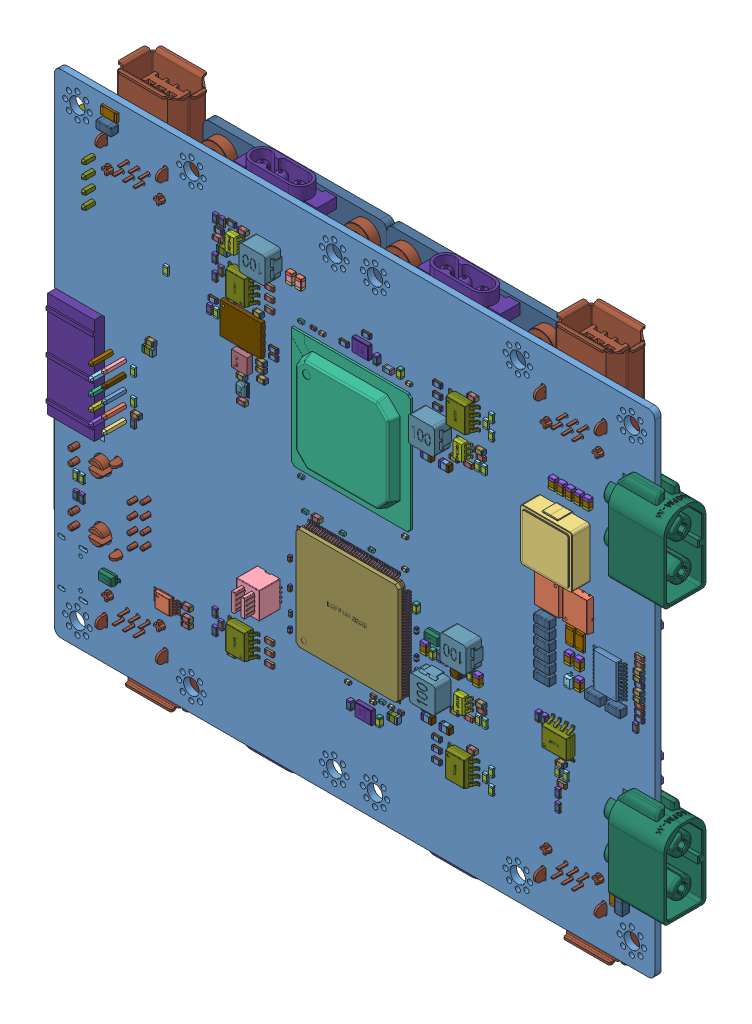
SolidWorks assembly Mother  Board, configuration 默认. Lengths in mm. (continued)
Components (placement in the parent): (continued)
- Mother  Board.step-1: Mother  Board.step [默认] at origin size (122.6 102.08 21) (continued)
  - Free-Models.step-1: Free-Models.step [默认] at origin size (70.87 98.07 8.62) (continued)
    - Driver_Board.step-4: Driver_Board.step [默认] at (21.971 0 -6.2) x (1 0 0) z (0 0 1) size (35.43 49.03 8.62) (continued)
      - R2.step-1: R2.step [默认] at origin size (0.8 1.6 0.45) (continued)
        - 6547515376.step-1: 6547515376.step [默认] at (-0.7621 21.0821 0) x (0 1 0) z (0 0 1) size (1.6 0.8 0.45) (continued)
          - Terminal-19.step-1: Terminal-19.step [默认] at (-0.8 -0.4 0) size (0.3 0.8 0.45)
            - Open_CASCADE_STEP_translator_6.8_21.2.1-76.step-1: Open_CASCADE_STEP_translator_6.8_21.2.1-76.step [默认] at origin size (0.3 0.8 0.45)
          - Terminal-19.step-2: Terminal-19.step [默认] at (0.8 0.4 0) x (-1 0 0) z (0 0 1) size (0.3 0.8 0.45)
            - Open_CASCADE_STEP_translator_6.8_21.2.1-76.step-1: Open_CASCADE_STEP_translator_6.8_21.2.1-76.step [默认] at origin size (0.3 0.8 0.45)
          - Mid_Body-77.step-1: Mid_Body-77.step [默认] at (-0.8 -0.4 0) size (1.51 0.8 0.36)
          - Mark-78.step-1: Mark-78.step [默认] at (-0.5 -0.4 0.405) size (1 0.8 0.05)
      - R1.step-1: R1.step [默认] at origin size (0.8 1.6 0.45)
        - 6547515376.step-1: 6547515376.step [默认] at (3.5559 13.5891 0) x (0 1 0) z (0 0 1) size (1.6 0.8 0.45)
          - Terminal-19.step-1: Terminal-19.step [默认] at (-0.8 -0.4 0) size (0.3 0.8 0.45)
            - Open_CASCADE_STEP_translator_6.8_21.2.1-76.step-1: Open_CASCADE_STEP_translator_6.8_21.2.1-76.step [默认] at origin size (0.3 0.8 0.45)
          - Terminal-19.step-2: Terminal-19.step [默认] at (0.8 0.4 0) x (-1 0 0) z (0 0 1) size (0.3 0.8 0.45)
            - Open_CASCADE_STEP_translator_6.8_21.2.1-76.step-1: Open_CASCADE_STEP_translator_6.8_21.2.1-76.step [默认] at origin size (0.3 0.8 0.45)
          - Mid_Body-77.step-1: Mid_Body-77.step [默认] at (-0.8 -0.4 0) size (1.51 0.8 0.36)
          - Mark-78.step-1: Mark-78.step [默认] at (-0.5 -0.4 0.405) size (1 0.8 0.05)
      - M6.step-1: M6.step [默认] at origin size (5.15 6.15 1.1)
        - TDSON-8-91.step-1: TDSON-8-91.step [默认] at (21.8441 12.7711 -1.6164) x (1 0 0) z (0 1 0) size (5.15 1.1 6.15)
      - M5.step-1: M5.step [默认] at origin size (5.15 6.15 1.1)
        - TDSON-8-91.step-1: TDSON-8-91.step [默认] at (27.3049 12.7713 -1.6164) x (-1 0 0) z (0 -1 0) size (5.15 1.1 6.15)
      - M4.step-1: M4.step [默认] at origin size (5.15 6.15 1.1)
        - TDSON-8-91.step-1: TDSON-8-91.step [默认] at (10.9221 15.0571 -1.6164) x (1 0 0) z (0 1 0) size (5.15 1.1 6.15)
      - M3.step-1: M3.step [默认] at origin size (5.15 6.15 1.1)
        - TDSON-8-91.step-1: TDSON-8-91.step [默认] at (16.3829 15.0573 -1.6164) x (-1 0 0) z (0 -1 0) size (5.15 1.1 6.15)
      - M2-1.step-1: M2-1.step [默认] at origin size (5.15 6.15 1.1)
        - TDSON-8-91.step-1: TDSON-8-91.step [默认] at (0 12.7711 -1.6164) x (1 0 0) z (0 1 0) size (5.15 1.1 6.15)
      - M1-1.step-1: M1-1.step [默认] at origin size (5.15 6.15 1.1)
        - TDSON-8-91.step-1: TDSON-8-91.step [默认] at (5.4609 12.7713 -1.6164) x (-1 0 0) z (0 -1 0) size (5.15 1.1 6.15)
      - JP4-1.step-1: JP4-1.step [默认] at origin size (5.56 5.56 4.53)
        - User_Library-SMTSO-M3-3ET.step-1: User_Library-SMTSO-M3-3ET.step [默认] at (27.5589 0.0001 -2.6164) x (0 0 1) z (0 1 0) size (4.53 5.56 5.56)
      - JP3-1.step-1: JP3-1.step [默认] at origin size (5.56 5.56 4.53)
        - User_Library-SMTSO-M3-3ET.step-1: User_Library-SMTSO-M3-3ET.step [默认] at (-0.0001 0.0001 -2.6164) x (0 0 1) z (0 1 0) size (4.53 5.56 5.56)
      - JP2.step-1: JP2.step [默认] at origin size (11.5 4.96 6.5)
        - SG340-GxxP-B1-2x12.step-1: SG340-GxxP-B1-2x12.step [默认] at (13.7793 38.9891 0) x (-1 0 0) z (0 0 1) size (11.5 4.96 6.5)
      - D3-1.step-1: D3-1.step [默认] at origin size (2.65 1.3 0.96)
        - SOD-323-1.step-1: SOD-323-1.step [默认] at (20.5836 25.1426 0.05) x (-1 0 0) z (0 0 1) size (2.65 1.3 0.96)
          - SOD-323-92.step-1: SOD-323-92.step [默认] at origin size (2.65 1.3 0.95)
          - LOGO______.__-93.step-1: LOGO______.__-93.step [默认] at (0.0033 0.0815 -0.003) x (-1 0 0) z (0 0 -1) size (0.9 1.04 0.01)
      - D2-1.step-1: D2-1.step [默认] at origin size (2.65 1.3 0.96)
        - SOD-323-1.step-1: SOD-323-1.step [默认] at (13.4716 25.1426 0.05) x (-1 0 0) z (0 0 1) size (2.65 1.3 0.96)
          - SOD-323-92.step-1: SOD-323-92.step [默认] at origin size (2.65 1.3 0.95)
          - LOGO______.__-93.step-1: LOGO______.__-93.step [默认] at (0.0033 0.0815 -0.003) x (-1 0 0) z (0 0 -1) size (0.9 1.04 0.01)
      - D1-1.step-1: D1-1.step [默认] at origin size (2.65 1.3 0.96)
        - SOD-323-1.step-1: SOD-323-1.step [默认] at (6.3596 25.1426 0.05) x (-1 0 0) z (0 0 1) size (2.65 1.3 0.96)
          - SOD-323-92.step-1: SOD-323-92.step [默认] at origin size (2.65 1.3 0.95)
          - LOGO______.__-93.step-1: LOGO______.__-93.step [默认] at (0.0033 0.0815 -0.003) x (-1 0 0) z (0 0 -1) size (0.9 1.04 0.01)
      - CP7-1.step-1: CP7-1.step [默认] at origin size (1.5 3 1.5)
        - (______)-94.step-1: (______)-94.step [默认] at (29.2101 17.1449 0) x (1 0 0) z (0 0 1) size (1.5 3 1.5)
      - CP9.step-1: CP9.step [默认] at origin size (1.5 3 1.5)
        - (______)-94.step-1: (______)-94.step [默认] at (18.2881 19.4309 0) x (1 0 0) z (0 0 1) size (1.5 3 1.5)
      - CP8-1.step-1: CP8-1.step [默认] at origin size (1.5 3 1.5)
        - (______)-94.step-1: (______)-94.step [默认] at (20.1931 19.4309 0) x (1 0 0) z (0 0 1) size (1.5 3 1.5)
      - CP5-1.step-1: CP5-1.step [默认] at origin size (1.5 3 1.5)
        - (______)-94.step-1: (______)-94.step [默认] at (9.3982 17.145 0) x (1 0 0) z (0 0 1) size (1.5 3 1.5)
      - CP4-1.step-1: CP4-1.step [默认] at origin size (1.5 3 1.5)
        - (______)-94.step-1: (______)-94.step [默认] at (7.4932 17.145 0) x (1 0 0) z (0 0 1) size (1.5 3 1.5)
      - CP3-1.step-1: CP3-1.step [默认] at origin size (1.5 3 1.5)
        - (______)-94.step-1: (______)-94.step [默认] at (27.3051 17.1449 0) x (1 0 0) z (0 0 1) size (1.5 3 1.5)
      - CP2-1.step-1: CP2-1.step [默认] at origin size (1.5 3 1.5)
        - (______)-94.step-1: (______)-94.step [默认] at (16.3831 19.4309 0) x (1 0 0) z (0 0 1) size (1.5 3 1.5)
      - CP1-1.step-1: CP1-1.step [默认] at origin size (1.5 3 1.5)
        - (______)-94.step-1: (______)-94.step [默认] at (5.5882 17.145 0) x (1 0 0) z (0 0 1) size (1.5 3 1.5)
      - C29-1.step-1: C29-1.step [默认] at origin size (1.6 0.8 0.8)
        - 6547515616.step-1: 6547515616.step [默认] at (22.9869 16.6369 0) x (-1 0 0) z (0 0 1) size (1.6 0.8 0.8)
          - Terminal-22.step-1: Terminal-22.step [默认] at (-0.8 -0.4 0) size (1.6 0.8 0.8)
            - Open_CASCADE_STEP_translator_6.8_47.1.1-85.step-1: Open_CASCADE_STEP_translator_6.8_47.1.1-85.step [默认] at origin size (0.3 0.8 0.8)
            - Open_CASCADE_STEP_translator_6.8_47.1.2-86.step-1: Open_CASCADE_STEP_translator_6.8_47.1.2-86.step [默认] at origin size (0.3 0.8 0.8)
          - Mid_Body-10.step-1: Mid_Body-10.step [默认] at (-0.8 -0.4 0) size (1 0.8 0.8)
            - Open_CASCADE_STEP_translator_6.8_47.2.1-87.step-1: Open_CASCADE_STEP_translator_6.8_47.2.1-87.step [默认] at origin size (1 0.8 0.8)
      - C28-1.step-1: C28-1.step [默认] at origin size (1.6 0.8 0.8)
        - 6547515616.step-1: 6547515616.step [默认] at (24.6379 10.6679 0) x (-1 0 0) z (0 0 1) size (1.6 0.8 0.8)
          - Terminal-22.step-1: Terminal-22.step [默认] at (-0.8 -0.4 0) size (1.6 0.8 0.8)
            - Open_CASCADE_STEP_translator_6.8_47.1.1-85.step-1: Open_CASCADE_STEP_translator_6.8_47.1.1-85.step [默认] at origin size (0.3 0.8 0.8)
            - Open_CASCADE_STEP_translator_6.8_47.1.2-86.step-1: Open_CASCADE_STEP_translator_6.8_47.1.2-86.step [默认] at origin size (0.3 0.8 0.8)
          - Mid_Body-10.step-1: Mid_Body-10.step [默认] at (-0.8 -0.4 0) size (1 0.8 0.8)
            - Open_CASCADE_STEP_translator_6.8_47.2.1-87.step-1: Open_CASCADE_STEP_translator_6.8_47.2.1-87.step [默认] at origin size (1 0.8 0.8)
      - C27-1.step-1: C27-1.step [默认] at origin size (2.01 1.25 0.94)
        - 6547513136.step-1: 6547513136.step [默认] at (20.8503 23.4725 0) x (-1 0 0) z (0 0 1) size (2.01 1.25 0.94)
          - Fillet1-95.step-1: Fillet1-95.step [默认] at origin size (0.5 1.25 0.94)
          - Fillet2-96.step-1: Fillet2-96.step [默认] at origin size (0.5 1.25 0.94)
          - body2-97.step-1: body2-97.step [默认] at origin size (1.01 1.22 0.92)
      - C26-1.step-1: C26-1.step [默认] at origin size (0.8 1.6 0.8)
        - 6547516096.step-1: 6547516096.step [默认] at (17.9295 24.7425 0) x (0 -1 0) z (0 0 1) size (1.6 0.8 0.8)
          - Terminal-23.step-1: Terminal-23.step [默认] at (-0.8 -0.4 0) size (1.6 0.8 0.8)
            - Open_CASCADE_STEP_translator_6.8_47.1.1-98.step-1: Open_CASCADE_STEP_translator_6.8_47.1.1-98.step [默认] at origin size (0.3 0.8 0.8)
            - Open_CASCADE_STEP_translator_6.8_47.1.2-99.step-1: Open_CASCADE_STEP_translator_6.8_47.1.2-99.step [默认] at origin size (0.3 0.8 0.8)
          - Mid_Body-11.step-1: Mid_Body-11.step [默认] at (-0.8 -0.4 0) size (1 0.8 0.8)
            - Open_CASCADE_STEP_translator_6.8_47.2.1-100.step-1: Open_CASCADE_STEP_translator_6.8_47.2.1-100.step [默认] at origin size (1 0.8 0.8)
      - C25-1.step-1: C25-1.step [默认] at origin size (1.25 2.01 0.94)
        - 6547514896.step-1: 6547514896.step [默认] at (23.5173 31.0126 0) x (0 1 0) z (0 0 1) size (2.01 1.25 0.94)
          - Fillet1-101.step-1: Fillet1-101.step [默认] at origin size (0.5 1.25 0.94)
          - Fillet2-102.step-1: Fillet2-102.step [默认] at origin size (0.5 1.25 0.94)
          - body2-103.step-1: body2-103.step [默认] at origin size (1.01 1.22 0.92)
      - C20-1.step-1: C20-1.step [默认] at origin size (1.6 0.8 0.8)
        - 6547515616.step-1: 6547515616.step [默认] at (12.0649 18.9229 0) x (-1 0 0) z (0 0 1) size (1.6 0.8 0.8)
          - Terminal-22.step-1: Terminal-22.step [默认] at (-0.8 -0.4 0) size (1.6 0.8 0.8)
            - Open_CASCADE_STEP_translator_6.8_47.1.1-85.step-1: Open_CASCADE_STEP_translator_6.8_47.1.1-85.step [默认] at origin size (0.3 0.8 0.8)
            - Open_CASCADE_STEP_translator_6.8_47.1.2-86.step-1: Open_CASCADE_STEP_translator_6.8_47.1.2-86.step [默认] at origin size (0.3 0.8 0.8)
          - Mid_Body-10.step-1: Mid_Body-10.step [默认] at (-0.8 -0.4 0) size (1 0.8 0.8)
            - Open_CASCADE_STEP_translator_6.8_47.2.1-87.step-1: Open_CASCADE_STEP_translator_6.8_47.2.1-87.step [默认] at origin size (1 0.8 0.8)
      - C19-1.step-1: C19-1.step [默认] at origin size (0.8 1.6 0.8)
        - 6547517776.step-1: 6547517776.step [默认] at (25.7809 37.7191 0) x (0 1 0) z (0 0 1) size (1.6 0.8 0.8)
          - Terminal-24.step-1: Terminal-24.step [默认] at (-0.8 -0.4 0) size (1.6 0.8 0.8)
            - Open_CASCADE_STEP_translator_6.8_47.1.1-104.step-1: Open_CASCADE_STEP_translator_6.8_47.1.1-104.step [默认] at origin size (0.3 0.8 0.8)
            - Open_CASCADE_STEP_translator_6.8_47.1.2-105.step-1: Open_CASCADE_STEP_translator_6.8_47.1.2-105.step [默认] at origin size (0.3 0.8 0.8)
          - Mid_Body-12.step-1: Mid_Body-12.step [默认] at (-0.8 -0.4 0) size (1 0.8 0.8)
            - Open_CASCADE_STEP_translator_6.8_47.2.1-106.step-1: Open_CASCADE_STEP_translator_6.8_47.2.1-106.step [默认] at origin size (1 0.8 0.8)
      - C18-1.step-1: C18-1.step [默认] at origin size (0.8 1.6 0.8)
        - 6547517776.step-1: 6547517776.step [默认] at (24.6379 37.7191 0) x (0 1 0) z (0 0 1) size (1.6 0.8 0.8)
          - Terminal-24.step-1: Terminal-24.step [默认] at (-0.8 -0.4 0) size (1.6 0.8 0.8)
            - Open_CASCADE_STEP_translator_6.8_47.1.1-104.step-1: Open_CASCADE_STEP_translator_6.8_47.1.1-104.step [默认] at origin size (0.3 0.8 0.8)
            - Open_CASCADE_STEP_translator_6.8_47.1.2-105.step-1: Open_CASCADE_STEP_translator_6.8_47.1.2-105.step [默认] at origin size (0.3 0.8 0.8)
          - Mid_Body-12.step-1: Mid_Body-12.step [默认] at (-0.8 -0.4 0) size (1 0.8 0.8)
            - Open_CASCADE_STEP_translator_6.8_47.2.1-106.step-1: Open_CASCADE_STEP_translator_6.8_47.2.1-106.step [默认] at origin size (1 0.8 0.8)
      - C17-1.step-1: C17-1.step [默认] at origin size (1.6 0.8 0.8)
        - 6547515616.step-1: 6547515616.step [默认] at (13.7159 12.9539 0) x (-1 0 0) z (0 0 1) size (1.6 0.8 0.8)
          - Terminal-22.step-1: Terminal-22.step [默认] at (-0.8 -0.4 0) size (1.6 0.8 0.8)
            - Open_CASCADE_STEP_translator_6.8_47.1.1-85.step-1: Open_CASCADE_STEP_translator_6.8_47.1.1-85.step [默认] at origin size (0.3 0.8 0.8)
            - Open_CASCADE_STEP_translator_6.8_47.1.2-86.step-1: Open_CASCADE_STEP_translator_6.8_47.1.2-86.step [默认] at origin size (0.3 0.8 0.8)
          - Mid_Body-10.step-1: Mid_Body-10.step [默认] at (-0.8 -0.4 0) size (1 0.8 0.8)
            - Open_CASCADE_STEP_translator_6.8_47.2.1-87.step-1: Open_CASCADE_STEP_translator_6.8_47.2.1-87.step [默认] at origin size (1 0.8 0.8)
      - C16-1.step-1: C16-1.step [默认] at origin size (0.8 1.6 0.8)
        - 6547516096.step-1: 6547516096.step [默认] at (25.7811 22.2249 0) x (0 -1 0) z (0 0 1) size (1.6 0.8 0.8)
          - Terminal-23.step-1: Terminal-23.step [默认] at (-0.8 -0.4 0) size (1.6 0.8 0.8)
            - Open_CASCADE_STEP_translator_6.8_47.1.1-98.step-1: Open_CASCADE_STEP_translator_6.8_47.1.1-98.step [默认] at origin size (0.3 0.8 0.8)
            - Open_CASCADE_STEP_translator_6.8_47.1.2-99.step-1: Open_CASCADE_STEP_translator_6.8_47.1.2-99.step [默认] at origin size (0.3 0.8 0.8)
          - Mid_Body-11.step-1: Mid_Body-11.step [默认] at (-0.8 -0.4 0) size (1 0.8 0.8)
            - Open_CASCADE_STEP_translator_6.8_47.2.1-100.step-1: Open_CASCADE_STEP_translator_6.8_47.2.1-100.step [默认] at origin size (1 0.8 0.8)
      - C15-1.step-1: C15-1.step [默认] at origin size (0.8 1.6 0.8)
        - 6547517776.step-1: 6547517776.step [默认] at (23.8759 25.6541 0) x (0 1 0) z (0 0 1) size (1.6 0.8 0.8)
          - Terminal-24.step-1: Terminal-24.step [默认] at (-0.8 -0.4 0) size (1.6 0.8 0.8)
            - Open_CASCADE_STEP_translator_6.8_47.1.1-104.step-1: Open_CASCADE_STEP_translator_6.8_47.1.1-104.step [默认] at origin size (0.3 0.8 0.8)
            - Open_CASCADE_STEP_translator_6.8_47.1.2-105.step-1: Open_CASCADE_STEP_translator_6.8_47.1.2-105.step [默认] at origin size (0.3 0.8 0.8)
          - Mid_Body-12.step-1: Mid_Body-12.step [默认] at (-0.8 -0.4 0) size (1 0.8 0.8)
            - Open_CASCADE_STEP_translator_6.8_47.2.1-106.step-1: Open_CASCADE_STEP_translator_6.8_47.2.1-106.step [默认] at origin size (1 0.8 0.8)
      - C14-1.step-1: C14-1.step [默认] at origin size (2.01 1.25 0.94)
        - 6547513136.step-1: 6547513136.step [默认] at (13.7383 23.4725 0) x (-1 0 0) z (0 0 1) size (2.01 1.25 0.94)
          - Fillet1-95.step-1: Fillet1-95.step [默认] at origin size (0.5 1.25 0.94)
          - Fillet2-96.step-1: Fillet2-96.step [默认] at origin size (0.5 1.25 0.94)
          - body2-97.step-1: body2-97.step [默认] at origin size (1.01 1.22 0.92)
      - C13-1.step-1: C13-1.step [默认] at origin size (0.8 1.6 0.8)
        - 6547516096.step-1: 6547516096.step [默认] at (10.8175 24.7425 0) x (0 -1 0) z (0 0 1) size (1.6 0.8 0.8)
          - Terminal-23.step-1: Terminal-23.step [默认] at (-0.8 -0.4 0) size (1.6 0.8 0.8)
            - Open_CASCADE_STEP_translator_6.8_47.1.1-98.step-1: Open_CASCADE_STEP_translator_6.8_47.1.1-98.step [默认] at origin size (0.3 0.8 0.8)
            - Open_CASCADE_STEP_translator_6.8_47.1.2-99.step-1: Open_CASCADE_STEP_translator_6.8_47.1.2-99.step [默认] at origin size (0.3 0.8 0.8)
          - Mid_Body-11.step-1: Mid_Body-11.step [默认] at (-0.8 -0.4 0) size (1 0.8 0.8)
            - Open_CASCADE_STEP_translator_6.8_47.2.1-100.step-1: Open_CASCADE_STEP_translator_6.8_47.2.1-100.step [默认] at origin size (1 0.8 0.8)
      - C12-1.step-1: C12-1.step [默认] at origin size (1.25 2.01 0.94)
        - 6547514896.step-1: 6547514896.step [默认] at (16.4053 31.0126 0) x (0 1 0) z (0 0 1) size (2.01 1.25 0.94)
          - Fillet1-101.step-1: Fillet1-101.step [默认] at origin size (0.5 1.25 0.94)
          - Fillet2-102.step-1: Fillet2-102.step [默认] at origin size (0.5 1.25 0.94)
          - body2-103.step-1: body2-103.step [默认] at origin size (1.01 1.22 0.92)
      - C11-1.step-1: C11-1.step [默认] at origin size (1.6 0.8 0.8)
        - 6547515616.step-1: 6547515616.step [默认] at (27.6859 22.8599 0) x (-1 0 0) z (0 0 1) size (1.6 0.8 0.8)
          - Terminal-22.step-1: Terminal-22.step [默认] at (-0.8 -0.4 0) size (1.6 0.8 0.8)
            - Open_CASCADE_STEP_translator_6.8_47.1.1-85.step-1: Open_CASCADE_STEP_translator_6.8_47.1.1-85.step [默认] at origin size (0.3 0.8 0.8)
            - Open_CASCADE_STEP_translator_6.8_47.1.2-86.step-1: Open_CASCADE_STEP_translator_6.8_47.1.2-86.step [默认] at origin size (0.3 0.8 0.8)
          - Mid_Body-10.step-1: Mid_Body-10.step [默认] at (-0.8 -0.4 0) size (1 0.8 0.8)
            - Open_CASCADE_STEP_translator_6.8_47.2.1-87.step-1: Open_CASCADE_STEP_translator_6.8_47.2.1-87.step [默认] at origin size (1 0.8 0.8)
      - C10-1.step-1: C10-1.step [默认] at origin size (0.8 1.6 0.8)
        - 6547517776.step-1: 6547517776.step [默认] at (-3.1751 37.7191 0) x (0 1 0) z (0 0 1) size (1.6 0.8 0.8)
          - Terminal-24.step-1: Terminal-24.step [默认] at (-0.8 -0.4 0) size (1.6 0.8 0.8)
            - Open_CASCADE_STEP_translator_6.8_47.1.1-104.step-1: Open_CASCADE_STEP_translator_6.8_47.1.1-104.step [默认] at origin size (0.3 0.8 0.8)
            - Open_CASCADE_STEP_translator_6.8_47.1.2-105.step-1: Open_CASCADE_STEP_translator_6.8_47.1.2-105.step [默认] at origin size (0.3 0.8 0.8)
          - Mid_Body-12.step-1: Mid_Body-12.step [默认] at (-0.8 -0.4 0) size (1 0.8 0.8)
            - Open_CASCADE_STEP_translator_6.8_47.2.1-106.step-1: Open_CASCADE_STEP_translator_6.8_47.2.1-106.step [默认] at origin size (1 0.8 0.8)
      - C9-1.step-1: C9-1.step [默认] at origin size (0.8 1.6 0.8)
        - 6547516096.step-1: 6547516096.step [默认] at (-3.1749 22.2249 0) x (0 -1 0) z (0 0 1) size (1.6 0.8 0.8)
          - Terminal-23.step-1: Terminal-23.step [默认] at (-0.8 -0.4 0) size (1.6 0.8 0.8)
            - Open_CASCADE_STEP_translator_6.8_47.1.1-98.step-1: Open_CASCADE_STEP_translator_6.8_47.1.1-98.step [默认] at origin size (0.3 0.8 0.8)
            - Open_CASCADE_STEP_translator_6.8_47.1.2-99.step-1: Open_CASCADE_STEP_translator_6.8_47.1.2-99.step [默认] at origin size (0.3 0.8 0.8)
          - Mid_Body-11.step-1: Mid_Body-11.step [默认] at (-0.8 -0.4 0) size (1 0.8 0.8)
            - Open_CASCADE_STEP_translator_6.8_47.2.1-100.step-1: Open_CASCADE_STEP_translator_6.8_47.2.1-100.step [默认] at origin size (1 0.8 0.8)
      - C8-1.step-1: C8-1.step [默认] at origin size (1.6 0.8 0.8)
        - 6547515616.step-1: 6547515616.step [默认] at (1.1429 16.5099 0) x (-1 0 0) z (0 0 1) size (1.6 0.8 0.8)
          - Terminal-22.step-1: Terminal-22.step [默认] at (-0.8 -0.4 0) size (1.6 0.8 0.8)
            - Open_CASCADE_STEP_translator_6.8_47.1.1-85.step-1: Open_CASCADE_STEP_translator_6.8_47.1.1-85.step [默认] at origin size (0.3 0.8 0.8)
            - Open_CASCADE_STEP_translator_6.8_47.1.2-86.step-1: Open_CASCADE_STEP_translator_6.8_47.1.2-86.step [默认] at origin size (0.3 0.8 0.8)
          - Mid_Body-10.step-1: Mid_Body-10.step [默认] at (-0.8 -0.4 0) size (1 0.8 0.8)
            - Open_CASCADE_STEP_translator_6.8_47.2.1-87.step-1: Open_CASCADE_STEP_translator_6.8_47.2.1-87.step [默认] at origin size (1 0.8 0.8)
      - C7-1.step-1: C7-1.step [默认] at origin size (0.8 1.6 0.8)
        - 6547516096.step-1: 6547516096.step [默认] at (-2.0319 22.2249 0) x (0 -1 0) z (0 0 1) size (1.6 0.8 0.8)
          - Terminal-23.step-1: Terminal-23.step [默认] at (-0.8 -0.4 0) size (1.6 0.8 0.8)
            - Open_CASCADE_STEP_translator_6.8_47.1.1-98.step-1: Open_CASCADE_STEP_translator_6.8_47.1.1-98.step [默认] at origin size (0.3 0.8 0.8)
            - Open_CASCADE_STEP_translator_6.8_47.1.2-99.step-1: Open_CASCADE_STEP_translator_6.8_47.1.2-99.step [默认] at origin size (0.3 0.8 0.8)
          - Mid_Body-11.step-1: Mid_Body-11.step [默认] at (-0.8 -0.4 0) size (1 0.8 0.8)
            - Open_CASCADE_STEP_translator_6.8_47.2.1-100.step-1: Open_CASCADE_STEP_translator_6.8_47.2.1-100.step [默认] at origin size (1 0.8 0.8)
      - C6-1.step-1: C6-1.step [默认] at origin size (0.8 1.6 0.8)
        - 6547517776.step-1: 6547517776.step [默认] at (-2.0321 37.7191 0) x (0 1 0) z (0 0 1) size (1.6 0.8 0.8)
          - Terminal-24.step-1: Terminal-24.step [默认] at (-0.8 -0.4 0) size (1.6 0.8 0.8)
            - Open_CASCADE_STEP_translator_6.8_47.1.1-104.step-1: Open_CASCADE_STEP_translator_6.8_47.1.1-104.step [默认] at origin size (0.3 0.8 0.8)
            - Open_CASCADE_STEP_translator_6.8_47.1.2-105.step-1: Open_CASCADE_STEP_translator_6.8_47.1.2-105.step [默认] at origin size (0.3 0.8 0.8)
          - Mid_Body-12.step-1: Mid_Body-12.step [默认] at (-0.8 -0.4 0) size (1 0.8 0.8)
            - Open_CASCADE_STEP_translator_6.8_47.2.1-106.step-1: Open_CASCADE_STEP_translator_6.8_47.2.1-106.step [默认] at origin size (1 0.8 0.8)
      - C5-1.step-1: C5-1.step [默认] at origin size (1.6 0.8 0.8)
        - 6547515616.step-1: 6547515616.step [默认] at (2.7939 10.6679 0) x (-1 0 0) z (0 0 1) size (1.6 0.8 0.8)
          - Terminal-22.step-1: Terminal-22.step [默认] at (-0.8 -0.4 0) size (1.6 0.8 0.8)
            - Open_CASCADE_STEP_translator_6.8_47.1.1-85.step-1: Open_CASCADE_STEP_translator_6.8_47.1.1-85.step [默认] at origin size (0.3 0.8 0.8)
            - Open_CASCADE_STEP_translator_6.8_47.1.2-86.step-1: Open_CASCADE_STEP_translator_6.8_47.1.2-86.step [默认] at origin size (0.3 0.8 0.8)
          - Mid_Body-10.step-1: Mid_Body-10.step [默认] at (-0.8 -0.4 0) size (1 0.8 0.8)
            - Open_CASCADE_STEP_translator_6.8_47.2.1-87.step-1: Open_CASCADE_STEP_translator_6.8_47.2.1-87.step [默认] at origin size (1 0.8 0.8)
      - C4-1.step-1: C4-1.step [默认] at origin size (1.6 0.8 0.8)
        - 6547515616.step-1: 6547515616.step [默认] at (-0.1271 22.8599 0) x (-1 0 0) z (0 0 1) size (1.6 0.8 0.8)
          - Terminal-22.step-1: Terminal-22.step [默认] at (-0.8 -0.4 0) size (1.6 0.8 0.8)
            - Open_CASCADE_STEP_translator_6.8_47.1.1-85.step-1: Open_CASCADE_STEP_translator_6.8_47.1.1-85.step [默认] at origin size (0.3 0.8 0.8)
            - Open_CASCADE_STEP_translator_6.8_47.1.2-86.step-1: Open_CASCADE_STEP_translator_6.8_47.1.2-86.step [默认] at origin size (0.3 0.8 0.8)
          - Mid_Body-10.step-1: Mid_Body-10.step [默认] at (-0.8 -0.4 0) size (1 0.8 0.8)
            - Open_CASCADE_STEP_translator_6.8_47.2.1-87.step-1: Open_CASCADE_STEP_translator_6.8_47.2.1-87.step [默认] at origin size (1 0.8 0.8)
      - C3-1.step-1: C3-1.step [默认] at origin size (2.01 1.25 0.94)
        - 6547513136.step-1: 6547513136.step [默认] at (6.6263 23.4725 0) x (-1 0 0) z (0 0 1) size (2.01 1.25 0.94)
          - Fillet1-95.step-1: Fillet1-95.step [默认] at origin size (0.5 1.25 0.94)
          - Fillet2-96.step-1: Fillet2-96.step [默认] at origin size (0.5 1.25 0.94)
          - body2-97.step-1: body2-97.step [默认] at origin size (1.01 1.22 0.92)
      - C2-1.step-1: C2-1.step [默认] at origin size (0.8 1.6 0.8)
        - 6547516096.step-1: 6547516096.step [默认] at (3.7055 24.7425 0) x (0 -1 0) z (0 0 1) size (1.6 0.8 0.8)
          - Terminal-23.step-1: Terminal-23.step [默认] at (-0.8 -0.4 0) size (1.6 0.8 0.8)
            - Open_CASCADE_STEP_translator_6.8_47.1.1-98.step-1: Open_CASCADE_STEP_translator_6.8_47.1.1-98.step [默认] at origin size (0.3 0.8 0.8)
            - Open_CASCADE_STEP_translator_6.8_47.1.2-99.step-1: Open_CASCADE_STEP_translator_6.8_47.1.2-99.step [默认] at origin size (0.3 0.8 0.8)
          - Mid_Body-11.step-1: Mid_Body-11.step [默认] at (-0.8 -0.4 0) size (1 0.8 0.8)
            - Open_CASCADE_STEP_translator_6.8_47.2.1-100.step-1: Open_CASCADE_STEP_translator_6.8_47.2.1-100.step [默认] at origin size (1 0.8 0.8)
      - C1.step-1: C1.step [默认] at origin size (1.25 2.01 0.94)
        - 6547514896.step-1: 6547514896.step [默认] at (9.2933 31.0126 0) x (0 1 0) z (0 0 1) size (2.01 1.25 0.94)
          - Fillet1-101.step-1: Fillet1-101.step [默认] at origin size (0.5 1.25 0.94)
          - Fillet2-102.step-1: Fillet2-102.step [默认] at origin size (0.5 1.25 0.94)
          - body2-103.step-1: body2-103.step [默认] at origin size (1.01 1.22 0.92)
